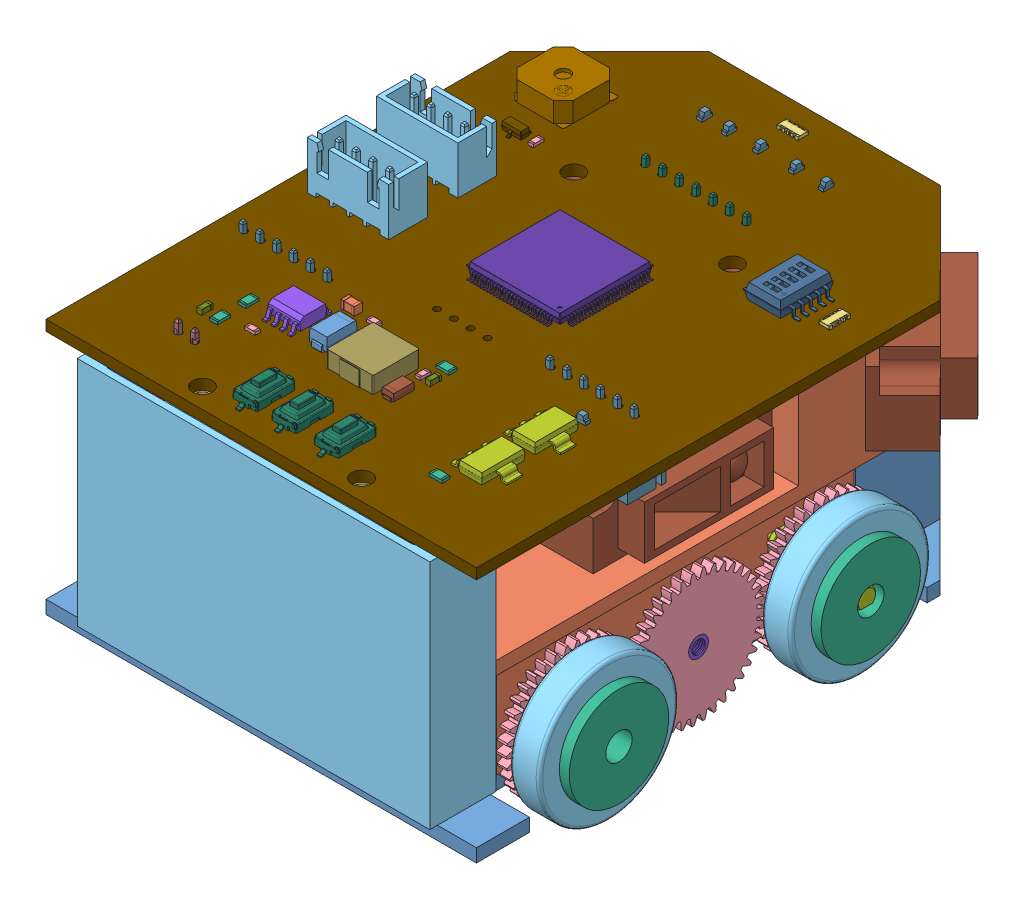
SolidWorks assembly ver 3.3, configuration Default. Lengths in mm.
Overall size (70 51.07 95.01).
215 component instances, 41 part files, 40 mates.
Components (placement in the parent):
- de 3.3-1: de 3.3 [Default] at (1.6493 45.7116 72.9223) size (64.97 15 85)
- cum banh 3.3-1: cum banh 3.3 [Default] at (-31.638 20.7951 90.3755) x (0 0 -1) z (1 0 0) size (61.3 24.42 40.4)
  - Ga Cum Banh 3.2-1: Ga Cum Banh 3.2 [Default] at (12.9532 31.9165 50.2873) size (60 15.5 15)
  - Bac lot-1: Bac lot [Default] at (-6.0468 31.9165 59.2873) size (9 9 6)
  - spur gear_iso-1: spur gear_iso [ISO - Spur gear 0.5M 38T 20PA 1.5FW ---S38A75H50L3.0N] at (12.9532 31.9165 61.2873) x (0 0 -1) z (1 0 0) size (1.5 19.95 20)
  - Lop banh xe-1: Lop banh xe [Default] at (-6.0468 31.9165 67.5373) x (0 0 -1) z (0.983863 -0.178922 0) size (4.5 21 21)
  - Mam banh xe-1: Mam banh xe [Default] at (-6.0468 31.9165 61.2873) x (-0.608419 -0.793616 0) z (0 0 -1) size (15 15 7)
  - N20 Mini Micro Metall Gear Motor DC 3-6-12V-1: N20 Mini Micro Metall Gear Motor DC 3-6-12V [Default] at (31.9532 31.9165 48.6873) x (0 0 1) z (-1 0 0) size (39.8 12.15 18.58)
  - spur gear_iso-2: spur gear_iso [ISO - Spur gear 0.5M 38T 20PA 1.5FW ---S38A75H50L3.0N] at (31.9532 31.9165 59.7873) x (0 0 1) z (-0.993186 0.116537 0) size (1.5 19.95 20)
  - spur gear_iso-3: spur gear_iso [ISO - Spur gear 0.5M 38T 20PA 1.5FW ---S38A75H50L3.0N] at (-6.0468 31.9165 61.2873) x (0 0 -1) z (1 0 0) size (1.5 19.95 20)
  - Bac lot-2: Bac lot [Default] at (12.9532 31.9165 59.2873) size (9 9 6)
  - Bac lot-3: Bac lot [Default] at (12.9532 31.9165 41.2873) x (0.064602 -0.997911 0) z (0 0 -1) size (9 9 6)
  - Bac lot-4: Bac lot [Default] at (-6.0468 31.9165 41.2873) x (-0.6399 -0.768458 0) z (0 0 -1) size (9 9 6)
  - Tru ren trong-1: Tru ren trong [Default] at (12.9532 31.9165 61.2873) x (0.857173 -0.515029 0) z (0 0 1) size (3 3 20.11)
  - Tru ren trong-2: Tru ren trong [Default] at (-6.0468 31.9165 61.2873) x (-0.86392 -0.50363 0) z (0 0 1) size (3 3 20.11)
  - Mam banh xe-2: Mam banh xe [Default] at (31.9532 31.9165 61.2873) x (-1 0 0) z (0 0 -1) size (15 15 7)
  - Lop banh xe-2: Lop banh xe [Default] at (31.9532 31.9165 67.5373) x (0 0 -1) z (1 0 0) size (4.5 21 21)
- cum banh 3.3-2: cum banh 3.3 [Default] at (34.9366 20.7951 64.4691) x (0 0 1) z (-1 0 0) size (61.3 24.42 40.4)
  - Ga Cum Banh 3.2-1: Ga Cum Banh 3.2 [Default] at (12.9532 31.9165 50.2873) size (60 15.5 15)
  - Bac lot-1: Bac lot [Default] at (-6.0468 31.9165 59.2873) size (9 9 6)
  - spur gear_iso-1: spur gear_iso [ISO - Spur gear 0.5M 38T 20PA 1.5FW ---S38A75H50L3.0N] at (12.9532 31.9165 61.2873) x (0 0 -1) z (1 0 0) size (1.5 19.95 20)
  - Lop banh xe-1: Lop banh xe [Default] at (-6.0468 31.9165 67.5373) x (0 0 -1) z (0.983863 -0.178922 0) size (4.5 21 21)
  - Mam banh xe-1: Mam banh xe [Default] at (-6.0468 31.9165 61.2873) x (-0.608419 -0.793616 0) z (0 0 -1) size (15 15 7)
  - N20 Mini Micro Metall Gear Motor DC 3-6-12V-1: N20 Mini Micro Metall Gear Motor DC 3-6-12V [Default] at (31.9532 31.9165 48.6873) x (0 0 1) z (-1 0 0) size (39.8 12.15 18.58)
  - spur gear_iso-2: spur gear_iso [ISO - Spur gear 0.5M 38T 20PA 1.5FW ---S38A75H50L3.0N] at (31.9532 31.9165 59.7873) x (0 0 1) z (-0.993186 0.116537 0) size (1.5 19.95 20)
  - spur gear_iso-3: spur gear_iso [ISO - Spur gear 0.5M 38T 20PA 1.5FW ---S38A75H50L3.0N] at (-6.0468 31.9165 61.2873) x (0 0 -1) z (1 0 0) size (1.5 19.95 20)
  - Bac lot-2: Bac lot [Default] at (12.9532 31.9165 59.2873) size (9 9 6)
  - Bac lot-3: Bac lot [Default] at (12.9532 31.9165 41.2873) x (0.064602 -0.997911 0) z (0 0 -1) size (9 9 6)
  - Bac lot-4: Bac lot [Default] at (-6.0468 31.9165 41.2873) x (-0.6399 -0.768458 0) z (0 0 -1) size (9 9 6)
  - Tru ren trong-1: Tru ren trong [Default] at (12.9532 31.9165 61.2873) x (0.857173 -0.515029 0) z (0 0 1) size (3 3 20.11)
  - Tru ren trong-2: Tru ren trong [Default] at (-6.0468 31.9165 61.2873) x (-0.86392 -0.50363 0) z (0 0 1) size (3 3 20.11)
  - Mam banh xe-2: Mam banh xe [Default] at (31.9532 31.9165 61.2873) x (-1 0 0) z (0 0 -1) size (15 15 7)
  - Lop banh xe-2: Lop banh xe [Default] at (31.9532 31.9165 67.5373) x (0 0 -1) z (1 0 0) size (4.5 21 21)
- pin7.4v 2000mAh 30C-1: pin7.4v 2000mAh 30C [Default] at (1.6493 67.7116 113.6223) x (1 0 0) z (0 1 0) size (19 73 16)
- GP2Y0A41SK0F-1: GP2Y0A41SK0F [Default] at (1.6493 51.9116 43.9223) x (1 0 0) z (0 0 -1) size (29.5 18.9 13.5)
- SHARP GP2Y0A51SK0F.step-2: SHARP GP2Y0A51SK0F.step [Default] at (-3.1733 50.5411 72.9409) x (0 0 -1) z (0 1 0) size (27 14.5 13.5)
  - шарп крышка.step-1: шарп крышка.step [Default] at (-12.8819 -17.3225 12.1705) x (1 0 0) z (0 -1 0) size (27 11 12)
  - шарп плата.step-1: шарп плата.step [Default] at (13.6181 -19.3225 25.6705) x (-1 0 0) z (0 -1 0) size (26 13 5.5)
  - 92000A010_Passivated 18-8 Stainless Steel Pan Head Phillips Screws.step-1: 92000A010_Passivated 18-8 Stainless Steel Pan Head Phillips Screws.step [Default] at (11.4181 -22.3225 19.1705) x (1 0 0) z (0 1 0) size (4 4 4.61)
  - 92000A010_Passivated 18-8 Stainless Steel Pan Head Phillips Screws.step-2: 92000A010_Passivated 18-8 Stainless Steel Pan Head Phillips Screws.step [Default] at (-10.1819 -22.3225 14.8705) x (1 0 0) z (0 1 0) size (4 4 4.61)
- SHARP GP2Y0A51SK0F.step-3: SHARP GP2Y0A51SK0F.step [Default] at (-1.0395 50.5411 51.4342) x (-0.708334 0 0.705877) z (0 1 0) size (27 14.5 13.5)
  - шарп крышка.step-1: шарп крышка.step [Default] at (-12.8819 -17.3225 12.1705) x (1 0 0) z (0 -1 0) size (27 11 12)
  - шарп плата.step-1: шарп плата.step [Default] at (13.6181 -19.3225 25.6705) x (-1 0 0) z (0 -1 0) size (26 13 5.5)
  - 92000A010_Passivated 18-8 Stainless Steel Pan Head Phillips Screws.step-1: 92000A010_Passivated 18-8 Stainless Steel Pan Head Phillips Screws.step [Default] at (11.4181 -22.3225 19.1705) x (1 0 0) z (0 1 0) size (4 4 4.61)
  - 92000A010_Passivated 18-8 Stainless Steel Pan Head Phillips Screws.step-2: 92000A010_Passivated 18-8 Stainless Steel Pan Head Phillips Screws.step [Default] at (-10.1819 -22.3225 14.8705) x (1 0 0) z (0 1 0) size (4 4 4.61)
- SHARP GP2Y0A51SK0F.step-4: SHARP GP2Y0A51SK0F.step [Default] at (6.4718 50.5411 71.7047) x (0 0 1) z (0 1 0) size (27 14.5 13.5)
  - шарп крышка.step-1: шарп крышка.step [Default] at (-12.8819 -17.3225 12.1705) x (1 0 0) z (0 -1 0) size (27 11 12)
  - шарп плата.step-1: шарп плата.step [Default] at (13.6181 -19.3225 25.6705) x (-1 0 0) z (0 -1 0) size (26 13 5.5)
  - 92000A010_Passivated 18-8 Stainless Steel Pan Head Phillips Screws.step-1: 92000A010_Passivated 18-8 Stainless Steel Pan Head Phillips Screws.step [Default] at (11.4181 -22.3225 19.1705) x (1 0 0) z (0 1 0) size (4 4 4.61)
  - 92000A010_Passivated 18-8 Stainless Steel Pan Head Phillips Screws.step-2: 92000A010_Passivated 18-8 Stainless Steel Pan Head Phillips Screws.step [Default] at (-10.1819 -22.3225 14.8705) x (1 0 0) z (0 1 0) size (4 4 4.61)
- SHARP GP2Y0A51SK0F.step-5: SHARP GP2Y0A51SK0F.step [Default] at (5.2247 50.5411 52.3032) x (-0.706112 0 -0.708101) z (0 1 0) size (27 14.5 13.5)
  - шарп крышка.step-1: шарп крышка.step [Default] at (-12.8819 -17.3225 12.1705) x (1 0 0) z (0 -1 0) size (27 11 12)
  - шарп плата.step-1: шарп плата.step [Default] at (13.6181 -19.3225 25.6705) x (-1 0 0) z (0 -1 0) size (26 13 5.5)
  - 92000A010_Passivated 18-8 Stainless Steel Pan Head Phillips Screws.step-1: 92000A010_Passivated 18-8 Stainless Steel Pan Head Phillips Screws.step [Default] at (11.4181 -22.3225 19.1705) x (1 0 0) z (0 1 0) size (4 4 4.61)
  - 92000A010_Passivated 18-8 Stainless Steel Pan Head Phillips Screws.step-2: 92000A010_Passivated 18-8 Stainless Steel Pan Head Phillips Screws.step [Default] at (-10.1819 -22.3225 14.8705) x (1 0 0) z (0 1 0) size (4 4 4.61)
- schematic (2).step-1: schematic (2).step [Default] at (-177.8512 82.7116 -18.3873) x (1 0 0.000071) z (0 1 0) size (64.97 85.02 16.13)
  - LED_0603_1608Metric.step-1: LED_0603_1608Metric.step [Default] at (188.7822 -57.8002 1.65) x (0 -1 0) z (0 0 1) size (1.6 0.8 1.1)
    - LED_0603_1608Metric-0.step-1: LED_0603_1608Metric-0.step [Default] at origin size (1.6 0.8 1.1)
  - SW_Tactile_SPST_NO_Straight_CK_PTS636Sx25SMTRLFS.step-1: SW_Tactile_SPST_NO_Straight_CK_PTS636Sx25SMTRLFS.step [Default] at (173.4 -127.275 1.65) x (0 1 0) z (0 0 1) size (8 3.7 2.55)
    - PTS636Sx25SMTRLFS.step-1: PTS636Sx25SMTRLFS.step [Default] at origin size (8 3.7 2.55)
  - C_0603_1608Metric.step-1: C_0603_1608Metric.step [Default] at (184.5722 -112.8754 1.65) x (0 1 0) z (0 0 1) size (1.6 0.8 0.8)
    - C_0603_1608Metric-1.step-1: C_0603_1608Metric-1.step [Default] at origin size (1.6 0.8 0.8)
  - LQFP-100_14x14mm_P0.5mm.step-1: LQFP-100_14x14mm_P0.5mm.step [Default] at (179.8 -89 1.65) x (-1 0 0) z (0 0 1) size (16 16 1.5)
    - LQFP_100_14x14mm_P05mm.step-1: LQFP_100_14x14mm_P05mm.step [Default] at origin size (16 16 1.5)
  - SOT-23.step-1: SOT-23.step [Default] at (158.1922 -74.0902 1.65) x (0 -1 0) z (0 0 1) size (2.5 3 1.2)
    - SOT_23.step-1: SOT_23.step [Default] at origin size (2.5 3 1.2)
  - C_0603_1608Metric.step-2: C_0603_1608Metric.step [Default] at (158 -120.8 1.65) x (0 -1 0) z (0 0 1) size (1.6 0.8 0.8)
    - C_0603_1608Metric-1.step-1: C_0603_1608Metric-1.step [Default] at origin size (1.6 0.8 0.8)
  - D_SMA.step-1: D_SMA.step [Default] at (171.575 -115 1.65) x (0 -1 0) z (0 0 1) size (5 2.7 2.22)
    - D_SMA-2.step-1: D_SMA-2.step [Default] at origin size (5 2.7 2.22)
  - C_0805_2012Metric.step-1: C_0805_2012Metric.step [Default] at (168.9622 -109.6002 1.65) size (2 1.25 1.25)
    - C_0805_2012Metric-3.step-1: C_0805_2012Metric-3.step [Default] at origin size (2 1.25 1.25)
  - LED_0603_1608Metric.step-2: LED_0603_1608Metric.step [Default] at (178.88 -57.7875 1.65) x (0 -1 0) z (0 0 1) size (1.6 0.8 1.1)
    - LED_0603_1608Metric-0.step-1: LED_0603_1608Metric-0.step [Default] at origin size (1.6 0.8 1.1)
  - R_Array_Convex_5x0603.step-1: R_Array_Convex_5x0603.step [Default] at (206.8422 -74.5602 1.65) x (-1 0 0) z (0 0 1) size (1.6 3.2 0.5)
    - R_Array_Convex_5x0603-4.step-1: R_Array_Convex_5x0603-4.step [Default] at origin size (1.6 3.2 0.5)
  - R_0603_1608Metric.step-1: R_0603_1608Metric.step [Default] at (161.05 -73.875 1.65) x (0 -1 0) z (0 0 1) size (1.6 0.8 0.45)
    - R_0603_1608Metric-5.step-1: R_0603_1608Metric-5.step [Default] at origin size (1.6 0.8 0.45)
  - R_0603_1608Metric.step-2: R_0603_1608Metric.step [Default] at (155.05 -78.75 1.65) x (0 -1 0) z (0 0 1) size (1.6 0.8 0.45)
    - R_0603_1608Metric-5.step-1: R_0603_1608Metric-5.step [Default] at origin size (1.6 0.8 0.45)
  - R_0603_1608Metric.step-3: R_0603_1608Metric.step [Default] at (157.65 -78.75 1.65) x (0 -1 0) z (0 0 1) size (1.6 0.8 0.45)
    - R_0603_1608Metric-5.step-1: R_0603_1608Metric-5.step [Default] at origin size (1.6 0.8 0.45)
  - JST - XH - Thru (V) - 4Pin - 2.54mm.step-1: JST - XH - Thru (V) - 4Pin - 2.54mm.step [Default] at (156.4 -95.1037 1.65) size (12.29 5.84 10.21)
    - JST - XH - Thru - 4Pin - 2.54mm.step-1: JST - XH - Thru - 4Pin - 2.54mm.step [Default] at origin size (12.29 5.84 10.21)
  - C_0603_1608Metric.step-3: C_0603_1608Metric.step [Default] at (169.0522 -114.6252 1.65) x (0 1 0) z (0 0 1) size (1.6 0.8 0.8)
    - C_0603_1608Metric-1.step-1: C_0603_1608Metric-1.step [Default] at origin size (1.6 0.8 0.8)
  - LED_0603_1608Metric.step-3: LED_0603_1608Metric.step [Default] at (184.2422 -57.7602 1.65) x (0 -1 0) z (0 0 1) size (1.6 0.8 1.1)
    - LED_0603_1608Metric-0.step-1: LED_0603_1608Metric-0.step [Default] at origin size (1.6 0.8 1.1)
  - R_0805_2012Metric.step-1: R_0805_2012Metric.step [Default] at (160.2 -116.4 1.65) x (0 1 0) z (0 0 1) size (2 1.2 0.45)
    - R_0805_2012Metric-6.step-1: R_0805_2012Metric-6.step [Default] at origin size (2 1.2 0.45)
  - JST - XH - Thru (V) - 4Pin - 2.54mm.step-2: JST - XH - Thru (V) - 4Pin - 2.54mm.step [Default] at (156.19 -83.5908 1.65) x (-1 0 0) z (0 0 1) size (12.29 5.84 10.21)
    - JST - XH - Thru - 4Pin - 2.54mm.step-1: JST - XH - Thru - 4Pin - 2.54mm.step [Default] at origin size (12.29 5.84 10.21)
  - R_0805_2012Metric.step-2: R_0805_2012Metric.step [Default] at (183.8822 -110.1902 1.65) x (-1 0 0) z (0 0 1) size (2 1.2 0.45)
    - R_0805_2012Metric-6.step-1: R_0805_2012Metric-6.step [Default] at origin size (2 1.2 0.45)
  - SOT-223.step-1: SOT-223.step [Default] at (200.0875 -119.57 1.65) size (7 6.5 1.7)
    - SOT_223.step-1: SOT_223.step [Default] at origin size (7 6.5 1.7)
  - SOT-223.step-2: SOT-223.step [Default] at (200.1422 -111.6002 1.65) size (7 6.5 1.7)
    - SOT_223.step-1: SOT_223.step [Default] at origin size (7 6.5 1.7)
  - R_0603_1608Metric.step-4: R_0603_1608Metric.step [Default] at (172.4222 -109.6502 1.65) size (1.6 0.8 0.45)
    - R_0603_1608Metric-5.step-1: R_0603_1608Metric-5.step [Default] at origin size (1.6 0.8 0.45)
  - LED_0603_1608Metric.step-4: LED_0603_1608Metric.step [Default] at (174.1622 -57.8202 1.65) x (0 -1 0) z (0 0 1) size (1.6 0.8 1.1)
    - LED_0603_1608Metric-0.step-1: LED_0603_1608Metric-0.step [Default] at origin size (1.6 0.8 1.1)
  - R_0805_2012Metric.step-3: R_0805_2012Metric.step [Default] at (160.2 -120.6875 1.65) x (0 1 0) z (0 0 1) size (2 1.2 0.45)
    - R_0805_2012Metric-6.step-1: R_0805_2012Metric-6.step [Default] at origin size (2 1.2 0.45)
  - R_Array_Convex_5x0603.step-2: R_Array_Convex_5x0603.step [Default] at (178.8922 -52.9602 1.65) x (0 1 0) z (0 0 1) size (1.6 3.2 0.5)
    - R_Array_Convex_5x0603-4.step-1: R_Array_Convex_5x0603-4.step [Default] at origin size (1.6 3.2 0.5)
  - SW_Tactile_SPST_NO_Straight_CK_PTS636Sx25SMTRLFS.step-2: SW_Tactile_SPST_NO_Straight_CK_PTS636Sx25SMTRLFS.step [Default] at (179.2 -127.2 1.65) x (0 1 0) z (0 0 1) size (8 3.7 2.55)
    - PTS636Sx25SMTRLFS.step-1: PTS636Sx25SMTRLFS.step [Default] at origin size (8 3.7 2.55)
  - SO-8_narrow_simple.step-1: SO-8_narrow_simple.step [Default] at (165.7508 -114.6 1.65) x (-1 0 0) z (0 0 1) size (4.8 6.2 2)
    - ASSEMBLY.step-1: ASSEMBLY.step [Default] at origin size (4.8 6.2 2)
  - SW_Tactile_SPST_NO_Straight_CK_PTS636Sx25SMTRLFS.step-3: SW_Tactile_SPST_NO_Straight_CK_PTS636Sx25SMTRLFS.step [Default] at (185.6 -127.2 1.65) x (0 1 0) z (0 0 1) size (8 3.7 2.55)
    - PTS636Sx25SMTRLFS.step-1: PTS636Sx25SMTRLFS.step [Default] at origin size (8 3.7 2.55)
  - LED_0603_1608Metric.step-5: LED_0603_1608Metric.step [Default] at (200.9422 -106.7002 1.65) x (-1 0 0) z (0 0 1) size (1.6 0.8 1.1)
    - LED_0603_1608Metric-0.step-1: LED_0603_1608Metric-0.step [Default] at origin size (1.6 0.8 1.1)
  - LED_0603_1608Metric.step-6: LED_0603_1608Metric.step [Default] at (170.4722 -57.8302 1.65) x (0 -1 0) z (0 0 1) size (1.6 0.8 1.1)
    - LED_0603_1608Metric-0.step-1: LED_0603_1608Metric-0.step [Default] at origin size (1.6 0.8 1.1)
  - GSC8530YA-16R2700.step-1: GSC8530YA-16R2700.step [Default] at (157.0222 -65.7202 1.65) x (-1 0 0) z (0 1 0) size (8.55 3.15 8.5)
    - GSC8530YA-16R2700-7.step-1: GSC8530YA-16R2700-7.step [Default] at origin size (8.55 3.15 8.5)
  - SW_DIP_SPSTx05_Slide_KingTek_DSHP05TS_W7.62mm_P1.27mm.step-1: SW_DIP_SPSTx05_Slide_KingTek_DSHP05TS_W7.62mm_P1.27mm.step [Default] at (200.1022 -74.7302 1.65) x (-1 0 0) z (0 0 1) size (8.35 7.95 2.38)
    - SW_DIP_SPSTx05_Slide_KingTek_DSHP05TS_W762mm_P127mm.step-1: SW_DIP_SPSTx05_Slide_KingTek_DSHP05TS_W762mm_P127mm.step [Default] at origin size (8.35 7.95 2.38)
  - R_0603_1608Metric.step-5: R_0603_1608Metric.step [Default] at (182.9722 -112.8652 1.65) x (0 1 0) z (0 0 1) size (1.6 0.8 0.45)
    - R_0603_1608Metric-5.step-1: R_0603_1608Metric-5.step [Default] at origin size (1.6 0.8 0.45)
  - R_0805_2012Metric.step-4: R_0805_2012Metric.step [Default] at (197.4675 -124.865 1.65) size (2 1.2 0.45)
    - R_0805_2012Metric-6.step-1: R_0805_2012Metric-6.step [Default] at origin size (2 1.2 0.45)
  - CP_EIA-3216-10_Kemet-I.step-1: CP_EIA-3216-10_Kemet-I.step [Default] at (183.3922 -117.0302 1.65) x (0 1 0) z (0 0 1) size (3.4 1.8 1.2)
    - CP_EIA_3216_10_Kemet_I.step-1: CP_EIA_3216_10_Kemet_I.step [Default] at origin size (3.4 1.8 1.2)
  - Inductor_7x7x2.5.step-1: Inductor_7x7x2.5.step [Default] at (178.1322 -115.5302 1.65) x (1 0 0) z (0 -1 0) size (7 2.6 7.2)
    - Inductor_7x7x2.5-8.step-1: Inductor_7x7x2.5-8.step [Default] at origin size (7 2.6 7.2)
  - R_0603_1608Metric.step-6: R_0603_1608Metric.step [Default] at (164.2 -119.8 1.65) x (-1 0 0) z (0 0 1) size (1.6 0.8 0.45)
    - R_0603_1608Metric-5.step-1: R_0603_1608Metric-5.step [Default] at origin size (1.6 0.8 0.45)
  - C_0603_1608Metric.step-4: C_0603_1608Metric.step [Default] at (195.3522 -91.7102 -0.05) x (1 0 0) z (0 0 -1) size (1.6 0.8 0.8)
    - C_0603_1608Metric-1.step-1: C_0603_1608Metric-1.step [Default] at origin size (1.6 0.8 0.8)
  - C_0603_1608Metric.step-5: C_0603_1608Metric.step [Default] at (180.3022 -85.9102 -0.05) x (-1 0 0) z (0 0 -1) size (1.6 0.8 0.8)
    - C_0603_1608Metric-1.step-1: C_0603_1608Metric-1.step [Default] at origin size (1.6 0.8 0.8)
  - C_0603_1608Metric.step-6: C_0603_1608Metric.step [Default] at (183.6572 -94.2302 -0.05) x (-1 0 0) z (0 0 -1) size (1.6 0.8 0.8)
    - C_0603_1608Metric-1.step-1: C_0603_1608Metric-1.step [Default] at origin size (1.6 0.8 0.8)
  - B2B-XH-A_LF__SN_.step-1: B2B-XH-A_LF__SN_.step [Default] at (159.9422 -124.9552 -0.05) x (-1 0 0) z (0 -1 0) size (7.4 10.4 5.75)
    - B2B-XH-A(LF)(SN).step-1: B2B-XH-A(LF)(SN).step [Default] at origin size (7.4 10.4 5.75)
  - R_0603_1608Metric.step-7: R_0603_1608Metric.step [Default] at (179.7 -125.6 -0.05) x (-1 0 0) z (0 0 -1) size (1.6 0.8 0.45)
    - R_0603_1608Metric-5.step-1: R_0603_1608Metric-5.step [Default] at origin size (1.6 0.8 0.45)
  - JST - XH - Thru (V) - 6Pin - 2.54mm.step-1: JST - XH - Thru (V) - 6Pin - 2.54mm.step [Default] at (197.6322 -101.9902 -0.05) x (1 0 0) z (0 0 -1) size (17.37 5.84 10.21)
    - JST - XH - Thru - 6Pin - 2.54mm.step-1: JST - XH - Thru - 6Pin - 2.54mm.step [Default] at origin size (17.37 5.84 10.21)
  - CP_EIA-3216-10_Kemet-I.step-2: CP_EIA-3216-10_Kemet-I.step [Default] at (201.5522 -117.3902 -0.05) x (1 0 0) z (0 0 -1) size (3.4 1.8 1.2)
    - CP_EIA_3216_10_Kemet_I.step-1: CP_EIA_3216_10_Kemet_I.step [Default] at origin size (3.4 1.8 1.2)
  - CP_EIA-3216-10_Kemet-I.step-3: CP_EIA-3216-10_Kemet-I.step [Default] at (177.2197 -105.6402 -0.05) x (-1 0 0) z (0 0 -1) size (3.4 1.8 1.2)
    - CP_EIA_3216_10_Kemet_I.step-1: CP_EIA_3216_10_Kemet_I.step [Default] at origin size (3.4 1.8 1.2)
  - R_0603_1608Metric.step-8: R_0603_1608Metric.step [Default] at (174.2 -125.475 -0.05) x (-1 0 0) z (0 0 -1) size (1.6 0.8 0.45)
    - R_0603_1608Metric-5.step-1: R_0603_1608Metric-5.step [Default] at origin size (1.6 0.8 0.45)
  - C_0603_1608Metric.step-7: C_0603_1608Metric.step [Default] at (183.6972 -92.4602 -0.05) x (-1 0 0) z (0 0 -1) size (1.6 0.8 0.8)
    - C_0603_1608Metric-1.step-1: C_0603_1608Metric-1.step [Default] at origin size (1.6 0.8 0.8)
  - CP_EIA-3216-10_Kemet-I.step-4: CP_EIA-3216-10_Kemet-I.step [Default] at (171.2722 -117.1002 -0.05) x (0 -1 0) z (0 0 -1) size (3.4 1.8 1.2)
    - CP_EIA_3216_10_Kemet_I.step-1: CP_EIA_3216_10_Kemet_I.step [Default] at origin size (3.4 1.8 1.2)
  - C_0603_1608Metric.step-8: C_0603_1608Metric.step [Default] at (184.8 -125.6 -0.05) x (1 0 0) z (0 0 -1) size (1.6 0.8 0.8)
    - C_0603_1608Metric-1.step-1: C_0603_1608Metric-1.step [Default] at origin size (1.6 0.8 0.8)
  - JST - XH - Thru (V) - 6Pin - 2.54mm.step-2: JST - XH - Thru (V) - 6Pin - 2.54mm.step [Default] at (156.6722 -107.3602 -0.05) x (1 0 0) z (0 0 -1) size (17.37 5.84 10.21)
    - JST - XH - Thru - 6Pin - 2.54mm.step-1: JST - XH - Thru - 6Pin - 2.54mm.step [Default] at origin size (17.37 5.84 10.21)
  - C_0603_1608Metric.step-9: C_0603_1608Metric.step [Default] at (177.5197 -107.4902 -0.05) x (-1 0 0) z (0 0 -1) size (1.6 0.8 0.8)
    - C_0603_1608Metric-1.step-1: C_0603_1608Metric-1.step [Default] at origin size (1.6 0.8 0.8)
  - JST - XH - Thru (V) - 7Pin - 2.54mm.step-1: JST - XH - Thru (V) - 7Pin - 2.54mm.step [Default] at (179.7522 -68.3802 -0.05) x (1 0 0) z (0 0 -1) size (19.91 5.84 10.21)
    - JST - XH - Thru - 7Pin - 2.54mm.step-1: JST - XH - Thru - 7Pin - 2.54mm.step [Default] at origin size (19.91 5.84 10.21)
  - C_0603_1608Metric.step-10: C_0603_1608Metric.step [Default] at (180.31 -87.58 -0.05) x (-1 0 0) z (0 0 -1) size (1.6 0.8 0.8)
    - C_0603_1608Metric-1.step-1: C_0603_1608Metric-1.step [Default] at origin size (1.6 0.8 0.8)
  - C_0603_1608Metric.step-11: C_0603_1608Metric.step [Default] at (183.6272 -88.9602 -0.05) x (-1 0 0) z (0 0 -1) size (1.6 0.8 0.8)
    - C_0603_1608Metric-1.step-1: C_0603_1608Metric-1.step [Default] at origin size (1.6 0.8 0.8)
  - CP_EIA-3216-10_Kemet-I.step-5: CP_EIA-3216-10_Kemet-I.step [Default] at (201.5422 -113.8002 -0.05) x (1 0 0) z (0 0 -1) size (3.4 1.8 1.2)
    - CP_EIA_3216_10_Kemet_I.step-1: CP_EIA_3216_10_Kemet_I.step [Default] at origin size (3.4 1.8 1.2)
  - R_0603_1608Metric.step-9: R_0603_1608Metric.step [Default] at (160.18 -91.9945 -0.05) x (0 1 0) z (0 0 -1) size (1.6 0.8 0.45)
    - R_0603_1608Metric-5.step-1: R_0603_1608Metric-5.step [Default] at origin size (1.6 0.8 0.45)
  - C_0603_1608Metric.step-12: C_0603_1608Metric.step [Default] at (183.5822 -85.8802 -0.05) x (1 0 0) z (0 0 -1) size (1.6 0.8 0.8)
    - C_0603_1608Metric-1.step-1: C_0603_1608Metric-1.step [Default] at origin size (1.6 0.8 0.8)
  - C_0603_1608Metric.step-13: C_0603_1608Metric.step [Default] at (175.4 -92.9 -0.05) x (1 0 0) z (0 0 -1) size (1.6 0.8 0.8)
    - C_0603_1608Metric-1.step-1: C_0603_1608Metric-1.step [Default] at origin size (1.6 0.8 0.8)
  - C_0603_1608Metric.step-14: C_0603_1608Metric.step [Default] at (195.4222 -86.5502 -0.05) x (1 0 0) z (0 0 -1) size (1.6 0.8 0.8)
    - C_0603_1608Metric-1.step-1: C_0603_1608Metric-1.step [Default] at origin size (1.6 0.8 0.8)
  - C_0603_1608Metric.step-15: C_0603_1608Metric.step [Default] at (183.6122 -84.1702 -0.05) x (1 0 0) z (0 0 -1) size (1.6 0.8 0.8)
    - C_0603_1608Metric-1.step-1: C_0603_1608Metric-1.step [Default] at origin size (1.6 0.8 0.8)
  - R_0603_1608Metric.step-10: R_0603_1608Metric.step [Default] at (200.5422 -109.4502 -0.05) x (-1 0 0) z (0 0 -1) size (1.6 0.8 0.45)
    - R_0603_1608Metric-5.step-1: R_0603_1608Metric-5.step [Default] at origin size (1.6 0.8 0.45)
  - Crystal_SMD_3225-4Pin_3.2x2.5mm.step-1: Crystal_SMD_3225-4Pin_3.2x2.5mm.step [Default] at (195.4222 -89.2002 -0.05) x (1 0 0) z (0 0 -1) size (3.2 2.5 0.64)
    - Crystal_SMD_3225-4Pin_3.2x2.5mm-9.step-1: Crystal_SMD_3225-4Pin_3.2x2.5mm-9.step [Default] at origin size (3.2 2.5 0.64)
  - C_0603_1608Metric.step-16: C_0603_1608Metric.step [Default] at (183.6 -82.6 -0.05) x (-1 0 0) z (0 0 -1) size (1.6 0.8 0.8)
    - C_0603_1608Metric-1.step-1: C_0603_1608Metric-1.step [Default] at origin size (1.6 0.8 0.8)
  - R_0603_1608Metric.step-11: R_0603_1608Metric.step [Default] at (157.68 -91.9445 -0.05) x (0 -1 0) z (0 0 -1) size (1.6 0.8 0.45)
    - R_0603_1608Metric-5.step-1: R_0603_1608Metric-5.step [Default] at origin size (1.6 0.8 0.45)
  - C_0603_1608Metric.step-17: C_0603_1608Metric.step [Default] at (179.7 -128.5 -0.05) x (-1 0 0) z (0 0 -1) size (1.6 0.8 0.8)
    - C_0603_1608Metric-1.step-1: C_0603_1608Metric-1.step [Default] at origin size (1.6 0.8 0.8)
  - R_0603_1608Metric.step-12: R_0603_1608Metric.step [Default] at (183.7 -97.3 -0.05) x (-1 0 0) z (0 0 -1) size (1.6 0.8 0.45)
    - R_0603_1608Metric-5.step-1: R_0603_1608Metric-5.step [Default] at origin size (1.6 0.8 0.45)
  - C_0603_1608Metric.step-18: C_0603_1608Metric.step [Default] at (174.2 -128.275 -0.05) x (-1 0 0) z (0 0 -1) size (1.6 0.8 0.8)
    - C_0603_1608Metric-1.step-1: C_0603_1608Metric-1.step [Default] at origin size (1.6 0.8 0.8)
  - C_0603_1608Metric.step-19: C_0603_1608Metric.step [Default] at (183.6 -90.7 -0.05) x (-1 0 0) z (0 0 -1) size (1.6 0.8 0.8)
    - C_0603_1608Metric-1.step-1: C_0603_1608Metric-1.step [Default] at origin size (1.6 0.8 0.8)
  - CP_EIA-3216-10_Kemet-I.step-6: CP_EIA-3216-10_Kemet-I.step [Default] at (201.5422 -111.5502 -0.05) x (1 0 0) z (0 0 -1) size (3.4 1.8 1.2)
    - CP_EIA_3216_10_Kemet_I.step-1: CP_EIA_3216_10_Kemet_I.step [Default] at origin size (3.4 1.8 1.2)
  - C_0603_1608Metric.step-20: C_0603_1608Metric.step [Default] at (152.48 -91.8945 -0.05) x (0 1 0) z (0 0 -1) size (1.6 0.8 0.8)
    - C_0603_1608Metric-1.step-1: C_0603_1608Metric-1.step [Default] at origin size (1.6 0.8 0.8)
  - C_0603_1608Metric.step-21: C_0603_1608Metric.step [Default] at (176.7 -85.4 -0.05) x (1 0 0) z (0 0 -1) size (1.6 0.8 0.8)
    - C_0603_1608Metric-1.step-1: C_0603_1608Metric-1.step [Default] at origin size (1.6 0.8 0.8)
  - C_0603_1608Metric.step-22: C_0603_1608Metric.step [Default] at (176.7 -83.7 -0.05) x (1 0 0) z (0 0 -1) size (1.6 0.8 0.8)
    - C_0603_1608Metric-1.step-1: C_0603_1608Metric-1.step [Default] at origin size (1.6 0.8 0.8)
  - C_0603_1608Metric.step-23: C_0603_1608Metric.step [Default] at (175.4 -94.5 -0.05) x (1 0 0) z (0 0 -1) size (1.6 0.8 0.8)
    - C_0603_1608Metric-1.step-1: C_0603_1608Metric-1.step [Default] at origin size (1.6 0.8 0.8)
  - CP_EIA-3216-10_Kemet-I.step-7: CP_EIA-3216-10_Kemet-I.step [Default] at (201.5375 -122.02 -0.05) x (1 0 0) z (0 0 -1) size (3.4 1.8 1.2)
    - CP_EIA_3216_10_Kemet_I.step-1: CP_EIA_3216_10_Kemet_I.step [Default] at origin size (3.4 1.8 1.2)
  - C_0603_1608Metric.step-24: C_0603_1608Metric.step [Default] at (173.1722 -116.6002 -0.05) x (0 -1 0) z (0 0 -1) size (1.6 0.8 0.8)
    - C_0603_1608Metric-1.step-1: C_0603_1608Metric-1.step [Default] at origin size (1.6 0.8 0.8)
  - SSOP-24_5.3x8.2mm_P0.65mm.step-1: SSOP-24_5.3x8.2mm_P0.65mm.step [Default] at (178.875 -116.225 -0.05) x (0 1 0) z (0 0 -1) size (7.8 8.2 2.1)
    - SSOP_24_53x82mm_P065mm.step-1: SSOP_24_53x82mm_P065mm.step [Default] at origin size (7.8 8.2 2.1)
  - schematic_PCB.step-1: schematic_PCB.step [Default] at origin size (64.97 85.02 1.6)
- ga 1-1: ga 1 [Default] at (1.6493 47.7116 42.9723) x (0 0 -1) z (1 0 0) size (8.85 13 37.6)
- ga 23-1: ga 23 [Default] at (1.6493 60.7116 104.4223) size (49 22 85.5)
- truc dong cai cai 30mm-1: truc dong cai cai 30mm [По умолчанию] at (-10.2505 62.7116 112.395) size (5 20 5.77)
- truc dong cai cai 30mm-3: truc dong cai cai 30mm [По умолчанию] at (13.7695 62.7116 112.3967) x (-0.942419 0 -0.334435) z (0.334435 0 -0.942419) size (5 20 5.77)
- ga pin-1: ga pin [Default] at (1.6493 59.7116 80.4223) x (0 0 -1) z (-1 0 0) size (70 12 15)
- ga duoi-1: ga duoi [Default] at (1.6493 47.7116 116.5788) size (53.2 35 10)
Mates (geometry in assembly coordinates):
- Coincident2: coincident anti-aligned: plane of de 3.3-1 through (1.6493 47.7116 72.9223) normal (0 1 0); plane of cum banh 3.3-2/Ga Cum Banh 3.2-1 through (-22.8507 47.7116 77.4223) normal (0 -1 0)
- Coincident3: coincident anti-aligned: plane of de 3.3-1 through (1.6493 47.7116 72.9223) normal (0 1 0); plane of cum banh 3.3-1/Ga Cum Banh 3.2-1 through (26.1493 47.7116 77.4223) normal (0 -1 0)
- Coincident6: coincident aligned: plane of cum banh 3.3-1/Ga Cum Banh 3.2-1 through (26.1493 52.7116 107.4223) normal (0 0 1); plane of cum banh 3.3-2/Ga Cum Banh 3.2-1 through (-22.8507 52.7116 107.4223) normal (0 0 1)
- Coincident8: coincident anti-aligned: plane of de 3.3-1 through (1.6493 47.7116 72.9223) normal (0 1 0); plane of GP2Y0A41SK0F-1 through (16.3993 47.7116 43.9223) normal (0 -1 0)
- Width2: width anti-aligned: plane of GP2Y0A41SK0F-1 through (16.3993 56.1116 43.9223) normal (1 0 0); plane of pin7.4v 2000mAh 30C-1 through (-13.1007 47.7116 43.9223) normal (-1 0 0); plane of GP2Y0A41SK0F-1 through (-7.8507 75.7116 40.6223) normal (-1 0 0); plane of pin7.4v 2000mAh 30C-1 through (11.1493 75.7116 40.6223) normal (1 0 0)
- Distance1: distance = 35 mm anti-aligned: plane of schematic (2).step-1/schematic_PCB.step-1 through (-177.8512 82.7116 -18.3873) normal (0 -1 0); plane of de 3.3-1 through (1.6493 47.7116 72.9223) normal (0 1 0)
- Coincident16: coincident aligned: plane of cum banh 3.3-1/Ga Cum Banh 3.2-1 through (26.1493 52.7116 77.4223) normal (1 0 0); plane of SHARP GP2Y0A51SK0F.step-2/шарп крышка.step-1 through (26.1493 68.2116 72.3228) normal (1 0 0)
- Coincident17: coincident aligned: plane of cum banh 3.3-2/Ga Cum Banh 3.2-1 through (-22.8507 52.7116 77.4223) normal (-1 0 0); plane of SHARP GP2Y0A51SK0F.step-4/шарп крышка.step-1 through (-22.8507 68.2116 72.3228) normal (-1 0 0)
- Coincident18: coincident aligned: plane of SHARP GP2Y0A51SK0F.step-2/шарп крышка.step-1 through (14.1493 73.7116 85.8228) normal (0 0 1); plane of SHARP GP2Y0A51SK0F.step-4/шарп крышка.step-1 through (-10.8507 62.7116 85.8228) normal (0 0 1)
- Coincident29: coincident aligned: plane of de 3.3-1 through (-33.3507 47.7116 30.4223) normal (0 0 -1); plane of GP2Y0A41SK0F-1 through (7.4493 51.9116 30.4223) normal (0 0 -1)
- Distance2: distance = 8 mm aligned: plane of de 3.3-1 through (-33.3507 47.7116 115.4223) normal (0 0 1); plane of cum banh 3.3-2/Ga Cum Banh 3.2-1 through (-22.8507 52.7116 107.4223) normal (0 0 1)
- Coincident30: coincident: point of de 3.3-1; plane of schematic (2).step-1/schematic_PCB.step-1 through (34.1293 82.7116 115.4223) normal (-0.000071 0 1)
- Width3: width aligned: plane of schematic (2).step-1/schematic_PCB.step-1 through (34.1343 82.7116 45.4323) normal (1 0 0.000071); plane of schematic (2).step-1/schematic_PCB.step-1 through (-30.8307 82.7116 115.4177) normal (-1 0 0.000071); plane of de 3.3-1 through (-30.8313 37.7116 107.4223) normal (-1 0 0); plane of de 3.3-1 through (34.1298 37.7116 107.4223) normal (1 0 0)
- Width4: width anti-aligned: plane of pin7.4v 2000mAh 30C-1 through (11.1493 75.7116 40.6223) normal (1 0 0); plane of pin7.4v 2000mAh 30C-1 through (-7.8507 75.7116 40.6223) normal (-1 0 0); plane of de 3.3-1 through (-30.8313 37.7116 107.4223) normal (-1 0 0); plane of de 3.3-1 through (34.1298 37.7116 107.4223) normal (1 0 0)
- Coincident33: coincident aligned: plane of de 3.3-1 through (26.1493 55.7116 47.4223) normal (1 0 0); plane of cum banh 3.3-1/Ga Cum Banh 3.2-1 through (26.1493 52.7116 77.4223) normal (1 0 0)
- Coincident34: coincident aligned: plane of de 3.3-1 through (-22.8507 55.7116 47.4223) normal (-1 0 0); plane of cum banh 3.3-2/Ga Cum Banh 3.2-1 through (-22.8507 52.7116 77.4223) normal (-1 0 0)
- Width5: width aligned: plane of ga 1-1 through (16.3993 47.7116 42.9723) normal (-1 0 0); plane of ga 1-1 through (-13.1007 47.7116 42.9723) normal (1 0 0); plane of GP2Y0A41SK0F-1 through (-13.1007 47.7116 43.9223) normal (-1 0 0); plane of GP2Y0A41SK0F-1 through (16.3993 56.1116 43.9223) normal (1 0 0)
- Coincident35: coincident anti-aligned: plane of de 3.3-1 through (1.6493 47.7116 72.9223) normal (0 1 0); plane of ga 1-1 through (-17.3507 47.7116 39.9723) normal (0 -1 0)
- Coincident36: coincident anti-aligned: plane of GP2Y0A41SK0F-1 through (-3.4007 56.1116 40.6223) normal (0 0 1); plane of ga 1-1 through (1.6493 50.7116 40.6223) normal (0 0 -1)
- Coincident37: coincident anti-aligned: plane of cum banh 3.3-1/Ga Cum Banh 3.2-1 through (26.1493 60.7116 77.4223) normal (0 1 0); plane of ga 23-1 through (1.6493 60.7116 104.4223) normal (0 -1 0)
- Coincident39: coincident aligned: plane of cum banh 3.3-1/Ga Cum Banh 3.2-1 through (26.1493 52.7116 77.4223) normal (1 0 0); plane of ga 23-1 through (26.1493 62.7116 104.4223) normal (1 0 0)
- Distance4: distance = 6 mm: point of SHARP GP2Y0A51SK0F.step-3/шарп крышка.step-1; plane of schematic (2).step-1/schematic_PCB.step-1 through (-15.8047 82.7116 30.3987) normal (0.000929 0 -1)
- Distance5: distance = 6 mm: point of SHARP GP2Y0A51SK0F.step-5/шарп крышка.step-1; plane of schematic (2).step-1/schematic_PCB.step-1 through (-15.8047 82.7116 30.3987) normal (0.000929 0 -1)
- Coincident43: coincident anti-aligned: plane of SHARP GP2Y0A51SK0F.step-2/шарп крышка.step-1 through (14.1493 62.7116 85.8228) normal (0 -1 0); plane of ga 23-1 through (1.6493 62.7116 104.4223) normal (0 1 0)
- Coincident44: coincident aligned: plane of SHARP GP2Y0A51SK0F.step-2/шарп крышка.step-1 through (14.1493 62.7116 85.8228) normal (0 -1 0); plane of SHARP GP2Y0A51SK0F.step-4/шарп крышка.step-1 through (-10.8507 62.7116 58.8228) normal (0 -1 0)
- Coincident45: coincident anti-aligned: plane of SHARP GP2Y0A51SK0F.step-3/шарп крышка.step-1 through (-4.1424 62.7116 30.071) normal (0 -1 0); plane of ga 23-1 through (1.6493 62.7116 104.4223) normal (0 1 0)
- Coincident46: coincident anti-aligned: plane of SHARP GP2Y0A51SK0F.step-5/шарп крышка.step-1 through (26.5869 62.7116 49.1933) normal (0 -1 0); plane of ga 23-1 through (1.6493 62.7116 104.4223) normal (0 1 0)
- Coincident47: coincident aligned: plane of SHARP GP2Y0A51SK0F.step-3/шарп крышка.step-1 through (-19.3519 68.2116 33.9337) normal (-0.705877 0 -0.708334); plane of schematic (2).step-1/schematic_PCB.step-1 through (-30.8357 82.7116 45.3777) normal (-0.705877 0 -0.708334)
- Coincident48: coincident aligned: plane of SHARP GP2Y0A51SK0F.step-5/шарп крышка.step-1 through (22.7192 68.2116 33.985) normal (0.708101 0 -0.706112); plane of schematic (2).step-1/schematic_PCB.step-1 through (19.1753 82.7116 30.4312) normal (0.708101 0 -0.706112)
- Coincident49: coincident aligned: plane of de 3.3-1 through (-33.3507 47.7116 115.4223) normal (0 0 1); plane of ga 23-1 through (11.1493 60.7116 115.4223) normal (0 0 1)
- Concentric1: concentric anti-aligned: cylinder of schematic (2).step-1/schematic_PCB.step-1 through (-10.2505 82.7116 112.395) axis (0 -1 0) radius 1.5003; cylinder of truc dong cai cai 30mm-1 through (-10.2505 82.7116 112.395) axis (0 1 0) radius 1.25
- Coincident51: coincident anti-aligned: plane of ga 23-1 through (1.6493 62.7116 104.4223) normal (0 1 0); plane of truc dong cai cai 30mm-1 through (-10.2505 62.7116 112.395) normal (0 -1 0)
- Concentric2: concentric anti-aligned: cylinder of schematic (2).step-1/schematic_PCB.step-1 through (13.7695 82.7116 112.3967) axis (0 -1 0) radius 1.5003; cylinder of truc dong cai cai 30mm-3 through (13.7695 82.7116 112.3967) axis (0 1 0) radius 1.25
- Coincident52: coincident anti-aligned: plane of ga 23-1 through (1.6493 62.7116 104.4223) normal (0 1 0); plane of truc dong cai cai 30mm-3 through (13.7695 62.7116 112.3967) normal (0 -1 0)
- Width6: width anti-aligned: plane of ga pin-1 through (-5.8507 58.7116 115.4223) normal (-1 0 0); plane of ga pin-1 through (9.1493 58.7116 115.4223) normal (1 0 0); plane of de 3.3-1 through (-7.8507 60.7116 115.4223) normal (1 0 0); plane of de 3.3-1 through (11.1493 60.7116 115.4223) normal (-1 0 0)
- Coincident54: coincident anti-aligned: plane of de 3.3-1 through (1.6493 47.7116 72.9223) normal (0 1 0); plane of ga pin-1 through (1.6493 47.7116 80.4223) normal (0 -1 0)
- Coincident55: coincident aligned: plane of de 3.3-1 through (-33.3507 47.7116 115.4223) normal (0 0 1); plane of ga pin-1 through (-5.8507 58.7116 115.4223) normal (0 0 1)
- Coincident56: coincident anti-aligned: plane of pin7.4v 2000mAh 30C-1 through (-7.8507 59.7116 40.6223) normal (0 -1 0); plane of ga pin-1 through (1.6493 59.7116 80.4223) normal (0 1 0)
- Coincident58: coincident anti-aligned: plane of de 3.3-1 through (1.6493 47.7116 72.9223) normal (0 1 0); plane of ga duoi-1 through (24.2493 47.7116 113.5788) normal (0 -1 0)
- Width7: width aligned: plane of ga duoi-1 through (-22.9507 82.7116 106.5788) normal (1 0 0); plane of de 3.3-1 through (26.2493 82.7116 106.5788) normal (-1 0 0); plane of ga duoi-1 through (26.1493 55.7116 47.4223) normal (1 0 0); plane of de 3.3-1 through (-22.8507 55.7116 47.4223) normal (-1 0 0)
